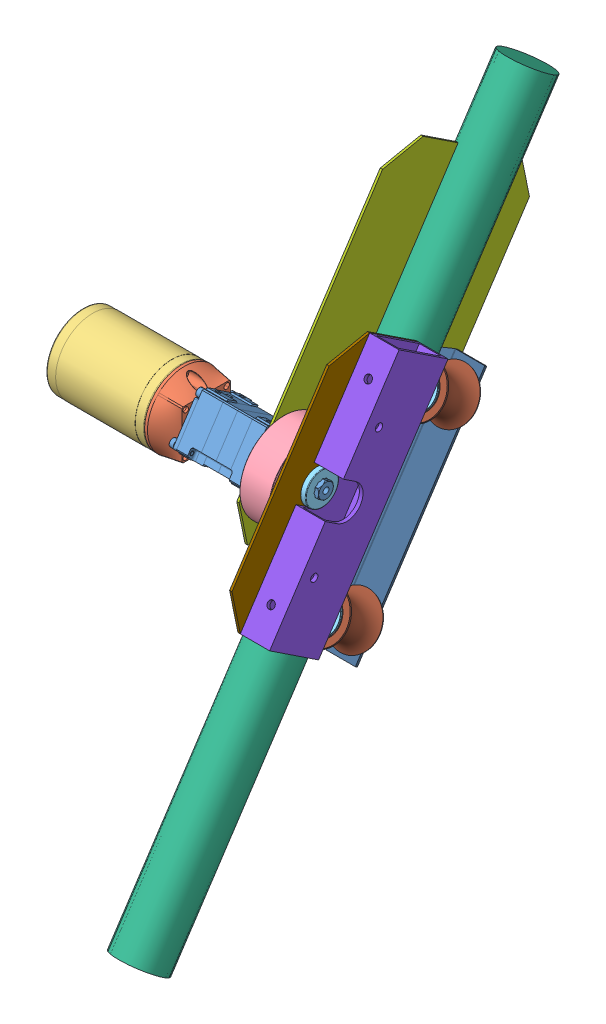
SolidWorks assembly ClimberWithPipe, configuration Default. Lengths in mm.
Overall size (242.1 535.26 382.45).
17 component instances, 11 part files, 0 mates.
Components (placement in the parent):
- ClimberWithPipe.stp-1: ClimberWithPipe.stp [Default] at origin size (242.1 535.26 382.45)
  - VersaPlanetary_v2_Two_Stage_100_1_with_BAG.stp-1: VersaPlanetary_v2_Two_Stage_100_1_with_BAG.stp [Default] at (-147.4647 -756.6918 -846.1082) x (1 0 0) z (0 0.551291 0.834313) size (110.6 44.45 42.65)
  - VersaPlanetary_CIM_Adapter_217-4018.stp-1: VersaPlanetary_CIM_Adapter_217-4018.stp [Default] at (-203.6897 -738.1492 -858.3607) x (0 -1 0) z (0 0 1) size (64.01 21.55 64.01)
  - Mini_CIM_Motor_217-3371.stp-1: Mini_CIM_Motor_217-3371.stp [Default] at (-215.2147 -738.1492 -858.3607) x (-1 0 0) z (0 0.447307 -0.894381) size (125.82 64.01 64.01)
  - am-3945 3IN 500Hex Compliant Wheel VER 3.stp-1: am-3945 3IN 500Hex Compliant Wheel VER 3.stp [Default] at (-85.5106 -746.8798 -917.1009) x (0 -0.212917 -0.97707) z (-1 0 0) size (76.2 76.2 25.4)
  - am-2986 FR8ZZ Hex Bearing.stp-1: am-2986 FR8ZZ Hex Bearing.stp [Default] at (-93.4483 -738.1492 -858.3607) x (0 0 1) z (-1 0 0) size (31.12 31.12 7.93)
  - Pipe.stp-1: Pipe.stp [Default] at (-120.4257 -787.3759 -894.767) x (0.159693 -0.544216 -0.823606) z (0 -0.834313 0.551291) size (42.16 42.16 609.6)
  - Bottom Wheel Plate.stp-1: Bottom Wheel Plate.stp [Default] at (-130.8397 -707.3598 -852.079) x (0 0.834313 -0.551291) z (1 0 0) size (275.87 152.4 2.03)
  - Top Bar.stp-1: Top Bar.stp [Default] at (-97.8197 -794.7225 -805.7565) x (0 -0.551291 -0.834313) z (1 0 0) size (50.8 203.2 25.4)
  - Top Wheel Plate.stp-1: Top Wheel Plate.stp [Default] at (-97.8197 -745.1506 -868.9565) x (0 0.551291 0.834313) z (-1 0 0) size (76.2 203.2 2.03)
  - am-2986 FR8ZZ Hex Bearing.stp-2: am-2986 FR8ZZ Hex Bearing.stp [Default] at (-85.1197 -827.0983 -854.7535) x (1 0 0) z (0 0.551291 0.834313) size (31.12 31.12 7.93)
  - am-2986 FR8ZZ Hex Bearing.stp-3: am-2986 FR8ZZ Hex Bearing.stp [Default] at (-85.1197 -699.949 -938.7703) x (1 0 0) z (0 0.551291 0.834313) size (31.12 31.12 7.93)
  - am-2986 FR8ZZ Hex Bearing.stp-4: am-2986 FR8ZZ Hex Bearing.stp [Default] at (-85.1197 -839.362 -873.3131) x (1 0 0) z (0 -0.551291 -0.834313) size (31.12 31.12 7.93)
  - am-2986 FR8ZZ Hex Bearing.stp-5: am-2986 FR8ZZ Hex Bearing.stp [Default] at (-85.1197 -712.2126 -957.3298) x (1 0 0) z (0 -0.551291 -0.834313) size (31.12 31.12 7.93)
  - Side Plate.stp-1: Side Plate.stp [Default] at (-69.5622 -843.7322 -879.927) x (1 0 0) z (0 -0.551291 -0.834313) size (100.44 203.2 15.23)
  - Roller.stp-1: Roller.stp [Default] at (-85.1197 -827.0983 -854.7535) x (-1 0 0) z (0 -0.551291 -0.834313) size (43.57 43.57 34.54)
  - Roller.stp-2: Roller.stp [Default] at (-85.1197 -699.949 -938.7703) x (-1 0 0) z (0 -0.551291 -0.834313) size (43.57 43.57 34.54)
